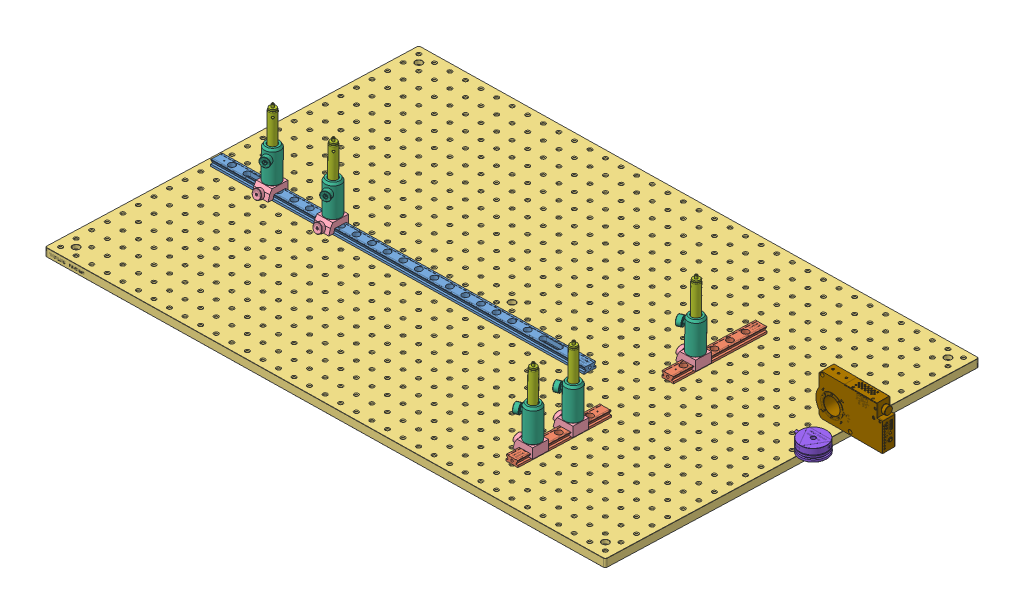
SolidWorks assembly OpenCALAssembly, configuration Default. Lengths in mm.
Overall size (1006.99 165.28 600.29).
31 component instances, 9 part files, 30 mates.
Components (placement in the parent):
- RLA600_M-Solidworks-1: RLA600_M-Solidworks [Default] at (212.74 428.5429 890.6377) x (0.000793 -0.03295 -0.999457) z (0.999847 0.01748 0.000217) size (19.05 9.53 600)
- RLA150_M-Solidworks-1: RLA150_M-Solidworks [Default] at (587.7819 430.9791 765.7872) x (0.999847 0.01748 0.000217) z (-0.000793 0.03295 0.999457) size (19.05 9.53 150)
- RLA150_M-Solidworks-2: RLA150_M-Solidworks [Default] at (587.5835 439.2167 1015.6513) x (-0.999847 -0.01748 -0.000217) z (0.000793 -0.03295 -0.999457) size (19.05 9.53 150)
- MB6090_M-Solidworks-1: MB6090_M-Solidworks [Default] at (350.5593 411.9431 853.774) x (0.999847 0.01748 0.000217) z (-0.000793 0.03295 0.999457) size (900 12.7 600)
- Rail-Post^OpenCALAssembly-1: Rail-Post^OpenCALAssembly [Default] at (243.8757 -121.8493 -138.0671) x (0.999969 -0.007878 0.000659) z (-0.000645 0.001893 0.999998) size (37.63 121.62 44.58) (virtual)
  - RC1-Solidworks-1: RC1-Solidworks [Default] at (-258.0543 541.4605 1048.8284) x (0.999678 0.025357 -0.000394) z (-0.000279 0.026514 0.999648) size (25.4 16.53 39.23)
  - socket head cap screw_am-1: socket head cap screw_am [B18.3.1M - 6 x 1.0 x 10 Hex SHCS -- 10NHX] at (-245.5045 547.2464 1029.7741) x (-0.025359 0.999327 -0.026513) z (0.026513 0.027184 0.999279) size (16 10 10)
  - PH50_M-Solidworks-1: PH50_M-Solidworks [Default] at (-244.0284 576.1062 1033.7923) x (0.926646 0.013547 -0.375692) z (0.37508 0.034095 0.926365) size (25 50.44 35.14)
  - TR75_M-Solidworks-1: TR75_M-Solidworks [Default] at (-246.3606 580.9852 1028.879) x (0.691707 -0.001607 -0.722176) z (0.721732 0.036653 0.691201) size (12.67 80.02 12.87)
- Rail-Post^OpenCALAssembly-2: Rail-Post^OpenCALAssembly [Default] at (341.3904 -120.1445 -138.0459) x (0.999969 -0.007878 0.000659) z (-0.000645 0.001893 0.999998) size (37.63 121.62 44.58) (virtual)
  - RC1-Solidworks-1: RC1-Solidworks [Default] at (-258.0543 541.4605 1048.8284) x (0.999678 0.025357 -0.000394) z (-0.000279 0.026514 0.999648) size (25.4 16.53 39.23)
  - socket head cap screw_am-1: socket head cap screw_am [B18.3.1M - 6 x 1.0 x 10 Hex SHCS -- 10NHX] at (-245.5045 547.2464 1029.7741) x (-0.025359 0.999327 -0.026513) z (0.026513 0.027184 0.999279) size (16 10 10)
  - PH50_M-Solidworks-1: PH50_M-Solidworks [Default] at (-244.0284 576.1062 1033.7923) x (0.926646 0.013547 -0.375692) z (0.37508 0.034095 0.926365) size (25 50.44 35.14)
  - TR75_M-Solidworks-1: TR75_M-Solidworks [Default] at (-246.3606 580.9852 1028.879) x (0.691707 -0.001607 -0.722176) z (0.721732 0.036653 0.691201) size (12.67 80.02 12.87)
- Rail-Post^OpenCALAssembly-4: Rail-Post^OpenCALAssembly [Default] at (1642.5862 -51.8881 1242.018) x (0.000044 0.007607 0.999971) z (-0.998822 -0.048519 0.000413) size (37.63 121.62 44.58) (virtual)
  - RC1-Solidworks-1: RC1-Solidworks [Default] at (-258.0543 541.4605 1048.8284) x (0.999678 0.025357 -0.000394) z (-0.000279 0.026514 0.999648) size (25.4 16.53 39.23)
  - socket head cap screw_am-1: socket head cap screw_am [B18.3.1M - 6 x 1.0 x 10 Hex SHCS -- 10NHX] at (-245.5045 547.2464 1029.7741) x (-0.025359 0.999327 -0.026513) z (0.026513 0.027184 0.999279) size (16 10 10)
  - PH50_M-Solidworks-1: PH50_M-Solidworks [Default] at (-244.0284 576.1062 1033.7923) x (0.926646 0.013547 -0.375692) z (0.37508 0.034095 0.926365) size (25 50.44 35.14)
  - TR75_M-Solidworks-1: TR75_M-Solidworks [Default] at (-246.3606 580.9852 1028.879) x (0.691707 -0.001607 -0.722176) z (0.721732 0.036653 0.691201) size (12.67 80.02 12.87)
- Rail-Post^OpenCALAssembly-6: Rail-Post^OpenCALAssembly [Default] at (1642.7424 -58.374 1045.2874) x (0.000044 0.007607 0.999971) z (-0.998822 -0.048519 0.000413) size (37.63 121.62 44.58) (virtual)
  - RC1-Solidworks-1: RC1-Solidworks [Default] at (-258.0543 541.4605 1048.8284) x (0.999678 0.025357 -0.000394) z (-0.000279 0.026514 0.999648) size (25.4 16.53 39.23)
  - socket head cap screw_am-1: socket head cap screw_am [B18.3.1M - 6 x 1.0 x 10 Hex SHCS -- 10NHX] at (-245.5045 547.2464 1029.7741) x (-0.025359 0.999327 -0.026513) z (0.026513 0.027184 0.999279) size (16 10 10)
  - PH50_M-Solidworks-1: PH50_M-Solidworks [Default] at (-244.0284 576.1062 1033.7923) x (0.926646 0.013547 -0.375692) z (0.37508 0.034095 0.926365) size (25 50.44 35.14)
  - TR75_M-Solidworks-1: TR75_M-Solidworks [Default] at (-246.3606 580.9852 1028.879) x (0.691707 -0.001607 -0.722176) z (0.721732 0.036653 0.691201) size (12.67 80.02 12.87)
- Rail-Post^OpenCALAssembly-8: Rail-Post^OpenCALAssembly [Default] at (1642.581 -49.6743 1306.6232) x (0.000044 0.007607 0.999971) z (-0.998822 -0.048519 0.000413) size (37.63 121.62 44.58) (virtual)
  - RC1-Solidworks-1: RC1-Solidworks [Default] at (-258.0543 541.4605 1048.8284) x (0.999678 0.025357 -0.000394) z (-0.000279 0.026514 0.999648) size (25.4 16.53 39.23)
  - socket head cap screw_am-1: socket head cap screw_am [B18.3.1M - 6 x 1.0 x 10 Hex SHCS -- 10NHX] at (-245.5045 547.2464 1029.7741) x (-0.025359 0.999327 -0.026513) z (0.026513 0.027184 0.999279) size (16 10 10)
  - PH50_M-Solidworks-1: PH50_M-Solidworks [Default] at (-244.0284 576.1062 1033.7923) x (0.926646 0.013547 -0.375692) z (0.37508 0.034095 0.926365) size (25 50.44 35.14)
  - TR75_M-Solidworks-1: TR75_M-Solidworks [Default] at (-246.3606 580.9852 1028.879) x (0.691707 -0.001607 -0.722176) z (0.721732 0.036653 0.691201) size (12.67 80.02 12.87)
- SB1-Solidworks-1: SB1-Solidworks [Default] at (818.5669 442.0324 849.7892) size (49.86 19.05 43.18)
- K10CR1_M-Solidworks-1: K10CR1_M-Solidworks [Default] at (824.7454 498.0338 801.9781) size (108.42 67.89 21.45)
Mates (geometry in assembly coordinates):
- Concentric5: concentric aligned: cylinder of RLA600_M-Solidworks-1 through (-62.2911 427.9239 890.4398) axis (-0.017463 0.999304 -0.032959) radius 3.3655; circle of MB6090_M-Solidworks-1
- Concentric6: concentric aligned: cylinder of RLA600_M-Solidworks-1 through (487.6248 437.538 890.5594) axis (-0.017463 0.999304 -0.032959) radius 3.3655; circle of MB6090_M-Solidworks-1
- Coincident8: coincident anti-aligned: plane of RLA600_M-Solidworks-1 through (512.7753 429.0243 900.3902) normal (0.017463 -0.999304 0.032959); plane of MB6090_M-Solidworks-1 through (-96.8299 426.6069 1150.0969) normal (-0.017463 0.999304 -0.032959)
- Coincident9: coincident anti-aligned: plane of RLA150_M-Solidworks-2 through (578.2082 431.5024 940.8575) normal (0.017463 -0.999304 0.032959); plane of MB6090_M-Solidworks-1 through (-96.8299 426.6069 1150.0969) normal (-0.017463 0.999304 -0.032959)
- Coincident10: coincident anti-aligned: plane of RLA150_M-Solidworks-1 through (597.3346 428.5404 840.9159) normal (0.017463 -0.999304 0.032959); plane of MB6090_M-Solidworks-1 through (-96.8299 426.6069 1150.0969) normal (-0.017463 0.999304 -0.032959)
- Concentric7: concentric aligned: cylinder of RLA600_M-Solidworks-1 through (-12.2988 428.7979 890.4507) axis (-0.017463 0.999304 -0.032959) radius 5.1562; cylinder of socket head cap screw_am-2 through (-200.2466 470.3352 1027.7075) axis (-0.025357 0.999196 -0.031056) radius 5
- Parallel5: parallel aligned: plane of RLA600_M-Solidworks-1 through (-87.2867 427.5323 884.1048) normal (-0.999847 -0.01748 -0.000217); plane of Rail-Post^OpenCALAssembly-1/RC1-Solidworks-1 through (-10.5574 422.7142 877.982) normal (-0.999847 -0.01748 -0.000217)
- Coincident23: coincident anti-aligned: plane of RLA600_M-Solidworks-1 through (512.6371 437.1668 881.4679) normal (0.009352 -0.524324 -0.851468); plane of Rail-Post^OpenCALAssembly-1/RC1-Solidworks-1 through (14.7938 425.6602 883.0857) normal (-0.009352 0.524324 0.851468)
- Parallel6: parallel aligned: plane of RLA600_M-Solidworks-1 through (-87.2867 427.5323 884.1048) normal (-0.999847 -0.01748 -0.000217); plane of Rail-Post^OpenCALAssembly-1/RC1-Solidworks-1 through (-10.5574 422.7142 877.982) normal (-0.999847 -0.01748 -0.000217)
- Coincident24: coincident: line of RLA600_M-Solidworks-1 through (512.6238 437.9283 881.4428) axis (-0.999847 -0.01748 -0.000217); plane of Rail-Post^OpenCALAssembly-1/RC1-Solidworks-1 through (14.7185 429.7567 900.0847) normal (0.017467 -0.999444 0.028416)
- Parallel7: parallel aligned: plane of RLA600_M-Solidworks-1 through (-87.2867 427.5323 884.1048) normal (-0.999847 -0.01748 -0.000217); plane of Rail-Post^OpenCALAssembly-2/RC1-Solidworks-1 through (86.9572 424.419 878.0032) normal (-0.999847 -0.01748 -0.000217)
- Coincident25: coincident anti-aligned: plane of RLA600_M-Solidworks-1 through (512.6371 437.1668 881.4679) normal (0.009352 -0.524324 -0.851468); plane of Rail-Post^OpenCALAssembly-2/RC1-Solidworks-1 through (112.3085 427.365 883.1069) normal (-0.009352 0.524324 0.851468)
- Parallel8: parallel aligned: plane of RLA600_M-Solidworks-1 through (-87.2867 427.5323 884.1048) normal (-0.999847 -0.01748 -0.000217); plane of Rail-Post^OpenCALAssembly-2/RC1-Solidworks-1 through (86.9572 424.419 878.0032) normal (-0.999847 -0.01748 -0.000217)
- Coincident26: coincident: line of RLA600_M-Solidworks-1 through (512.6238 437.9283 881.4428) axis (-0.999847 -0.01748 -0.000217); plane of Rail-Post^OpenCALAssembly-2/RC1-Solidworks-1 through (112.2332 431.4615 900.1059) normal (0.017467 -0.999444 0.028416)
- Parallel11: parallel aligned: plane of RLA150_M-Solidworks-2 through (581.2418 441.0767 940.5442) normal (0.000793 -0.03295 -0.999457); plane of Rail-Post^OpenCALAssembly-4/RC1-Solidworks-1 through (600.2998 436.7637 980.2933) normal (0.000793 -0.03295 -0.999457)
- Coincident29: coincident anti-aligned: plane of RLA150_M-Solidworks-2 through (596.6959 440.5852 940.5727) normal (0.876819 -0.480535 0.016538); plane of Rail-Post^OpenCALAssembly-4/RC1-Solidworks-1 through (595.0618 439.8415 1005.6015) normal (-0.876819 0.480535 -0.016538)
- Parallel12: parallel aligned: plane of RLA150_M-Solidworks-2 through (581.2418 441.0767 940.5442) normal (0.000793 -0.03295 -0.999457); plane of Rail-Post^OpenCALAssembly-4/RC1-Solidworks-1 through (600.2998 436.7637 980.2933) normal (0.000793 -0.03295 -0.999457)
- Coincident30: coincident: line of RLA150_M-Solidworks-2 through (596.6826 441.3467 940.5476) axis (-0.000793 0.03295 0.999457); plane of Rail-Post^OpenCALAssembly-4/RC1-Solidworks-1 through (577.8779 443.0744 1005.4813) normal (0.022008 -0.999214 0.03296)
- Concentric13: concentric anti-aligned: cylinder of RLA150_M-Solidworks-2 through (587.55 441.7572 965.5404) axis (-0.017463 0.999304 -0.032959) radius 5.1562; cone of MB6090_M-Solidworks-1 through (587.7119 432.4927 965.8459) axis (0.017463 -0.999304 0.032959)
- Concentric14: concentric anti-aligned: cylinder of RLA150_M-Solidworks-2 through (587.4707 445.0522 1065.4861) axis (-0.017463 0.999304 -0.032959) radius 5.1562; cone of MB6090_M-Solidworks-1 through (587.6326 435.7877 1065.7916) axis (0.017463 -0.999304 0.032959)
- Concentric15: concentric anti-aligned: cylinder of RLA150_M-Solidworks-1 through (587.669 436.8147 815.6219) axis (-0.017463 0.999304 -0.032959) radius 3.3655; cone of MB6090_M-Solidworks-1 through (587.8309 427.5501 815.9274) axis (0.017463 -0.999304 0.032959)
- Concentric16: concentric anti-aligned: cylinder of RLA150_M-Solidworks-1 through (587.7484 433.5197 715.6762) axis (-0.017463 0.999304 -0.032959) radius 5.1562; cone of MB6090_M-Solidworks-1 through (587.9103 424.2551 715.9818) axis (0.017463 -0.999304 0.032959)
- Parallel13: parallel aligned: plane of RLA150_M-Solidworks-2 through (581.2418 441.0767 940.5442) normal (0.000793 -0.03295 -0.999457); plane of Rail-Post^OpenCALAssembly-6/RC1-Solidworks-1 through (600.456 430.2779 783.5628) normal (0.000793 -0.03295 -0.999457)
- Coincident31: coincident anti-aligned: plane of RLA150_M-Solidworks-2 through (596.6959 440.5852 940.5727) normal (0.876819 -0.480535 0.016538); plane of Rail-Post^OpenCALAssembly-6/RC1-Solidworks-1 through (595.218 433.3557 808.8709) normal (-0.876819 0.480535 -0.016538)
- Parallel14: parallel aligned: plane of RLA150_M-Solidworks-2 through (581.2418 441.0767 940.5442) normal (0.000793 -0.03295 -0.999457); plane of Rail-Post^OpenCALAssembly-6/RC1-Solidworks-1 through (600.456 430.2779 783.5628) normal (0.000793 -0.03295 -0.999457)
- Coincident32: coincident: line of RLA150_M-Solidworks-2 through (596.6826 441.3467 940.5476) axis (-0.000793 0.03295 0.999457); plane of Rail-Post^OpenCALAssembly-6/RC1-Solidworks-1 through (578.0341 436.5886 808.7507) normal (0.022008 -0.999214 0.03296)
- Parallel17: parallel anti-aligned: plane of RLA150_M-Solidworks-1 through (593.9684 438.0028 840.6013) normal (-0.000793 0.03295 0.999457); plane of Rail-Post^OpenCALAssembly-8/RC1-Solidworks-1 through (600.2946 438.9776 1044.8985) normal (0.000793 -0.03295 -0.999457)
- Coincident35: coincident anti-aligned: plane of RLA150_M-Solidworks-1 through (596.7753 437.2902 840.627) normal (0.876819 -0.480535 0.016538); plane of Rail-Post^OpenCALAssembly-8/RC1-Solidworks-1 through (595.0565 442.0554 1070.2067) normal (-0.876819 0.480535 -0.016538)
- Parallel18: parallel aligned: plane of RLA150_M-Solidworks-1 through (594.0874 433.0603 690.6828) normal (0.000793 -0.03295 -0.999457); plane of Rail-Post^OpenCALAssembly-8/RC1-Solidworks-1 through (600.2946 438.9776 1044.8985) normal (0.000793 -0.03295 -0.999457)
- Coincident36: coincident: line of RLA150_M-Solidworks-1 through (578.5276 437.7329 840.5979) axis (0.000793 -0.03295 -0.999457); plane of Rail-Post^OpenCALAssembly-8/RC1-Solidworks-1 through (577.8727 445.2883 1070.0864) normal (0.022008 -0.999214 0.03296)
